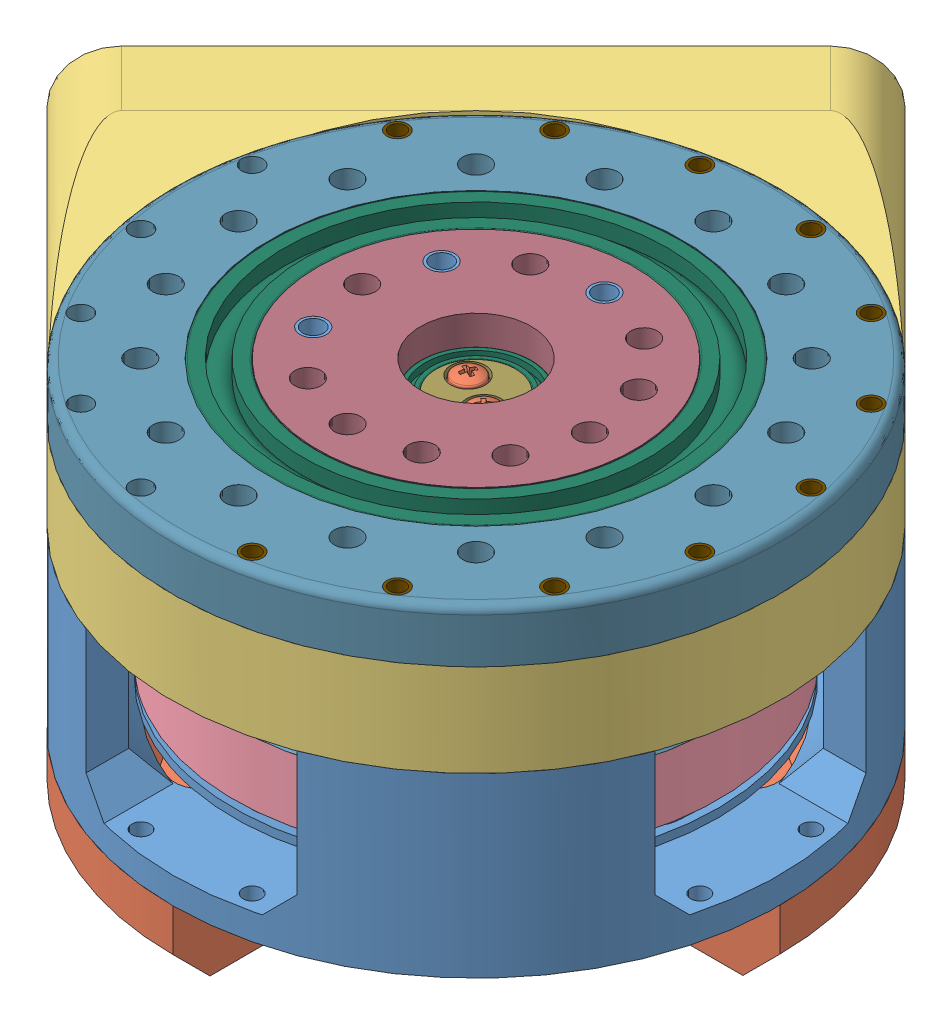
SolidWorks assembly Cycloidal_v2, configuration Default. Lengths in mm. (continued)
Components (placement in the parent): (continued)
- hex nut style 1 gradeab_iso-1: hex nut style 1 gradeab_iso [ISO - 4032 - M3 - W - N] at (47.267 33.7573 119.5643) x (1 0 0) z (0 -1 0) size (5.5 6.35 2.4)
- Cycloidal_Discs_8308-1: Cycloidal_Discs_8308 [Default] at (46.2249 42.227 18.2882) x (0.848672 0 0.528919) z (-0.528919 0 0.848672) size (79.25 5 79.73)
  - Cycloidal_Discs-1: Cycloidal_Discs [Default] at (38.3081 39.5303 58.0959) size (79.25 5 79.73)
  - radial ball bearing_68_iso-1: radial ball bearing_68_iso [ISO 15 RBB - 274 - 14,SI,NC,14_68] at (18.3896 43.2803 46.5959) x (0 1 0) z (0 0 1) size (2.5 7 7)
  - radial ball bearing_68_iso-2: radial ball bearing_68_iso [ISO 15 RBB - 274 - 14,SI,NC,14_68] at (38.3081 43.2803 81.0959) x (0 1 0) z (0 0 1) size (2.5 7 7)
  - radial ball bearing_68_iso-3: radial ball bearing_68_iso [ISO 15 RBB - 274 - 14,SI,NC,14_68] at (18.3896 43.2803 69.5959) x (0 1 0) z (0 0 1) size (2.5 7 7)
  - radial ball bearing_68_iso-4: radial ball bearing_68_iso [ISO 15 RBB - 274 - 14,SI,NC,14_68] at (38.3081 43.2803 35.0959) x (0 1 0) z (0 0 1) size (2.5 7 7)
  - radial ball bearing_68_iso-5: radial ball bearing_68_iso [ISO 15 RBB - 274 - 14,SI,NC,14_68] at (58.2267 43.2803 69.5959) x (0 1 0) z (0 0 1) size (2.5 7 7)
  - radial ball bearing_68_iso-6: radial ball bearing_68_iso [ISO 15 RBB - 274 - 14,SI,NC,14_68] at (58.2267 43.2803 46.5959) x (0 1 0) z (0 0 1) size (2.5 7 7)
- Cycloidal_Discs_8308-2: Cycloidal_Discs_8308 [Default] at (109.8312 37.227 61.5646) x (-0.154095 0 0.988056) z (-0.988056 0 -0.154095) size (79.25 5 79.73)
  - Cycloidal_Discs-1: Cycloidal_Discs [Default] at (38.3081 39.5303 58.0959) size (79.25 5 79.73)
  - radial ball bearing_68_iso-1: radial ball bearing_68_iso [ISO 15 RBB - 274 - 14,SI,NC,14_68] at (18.3896 43.2803 46.5959) x (0 1 0) z (0 0 1) size (2.5 7 7)
  - radial ball bearing_68_iso-2: radial ball bearing_68_iso [ISO 15 RBB - 274 - 14,SI,NC,14_68] at (38.3081 43.2803 81.0959) x (0 1 0) z (0 0 1) size (2.5 7 7)
  - radial ball bearing_68_iso-3: radial ball bearing_68_iso [ISO 15 RBB - 274 - 14,SI,NC,14_68] at (18.3896 43.2803 69.5959) x (0 1 0) z (0 0 1) size (2.5 7 7)
  - radial ball bearing_68_iso-4: radial ball bearing_68_iso [ISO 15 RBB - 274 - 14,SI,NC,14_68] at (38.3081 43.2803 35.0959) x (0 1 0) z (0 0 1) size (2.5 7 7)
  - radial ball bearing_68_iso-5: radial ball bearing_68_iso [ISO 15 RBB - 274 - 14,SI,NC,14_68] at (58.2267 43.2803 69.5959) x (0 1 0) z (0 0 1) size (2.5 7 7)
  - radial ball bearing_68_iso-6: radial ball bearing_68_iso [ISO 15 RBB - 274 - 14,SI,NC,14_68] at (58.2267 43.2803 46.5959) x (0 1 0) z (0 0 1) size (2.5 7 7)
- m6-1: m6 [Default] at (24.3083 92.633 87.7803) x (0 0 -1) z (-1 0 0) size (6 16 6)
- Motor_Cover_v2-2: Motor_Cover_v2 [Default] at (47.267 36.1573 89.1587) x (-1 0 0) z (0 0 -1) size (115 33.6 115)
- driver_cover-1: driver_cover [Default] at (47.267 36.1573 89.1587) x (-0.70834 0 -0.705872) z (-0.705872 0 0.70834) size (81.32 15 115)
- Base_plate_2 _new-1: Base_plate_2 _new [Default] at (47.267 69.6573 89.1587) x (-0.707107 0 0.707107) z (-0.707107 0 -0.707107) size (115 87.5 130)
Mates (geometry in assembly coordinates):
- Coincident1: coincident anti-aligned: plane of motor-X83008S.stp-1/outrunner.stp-1 through (64.3082 69.7573 59.1612) normal (0 1 0); plane of Base_Plate-1 through (47.267 69.7573 89.1587) normal (0 -1 0)
- Concentric1: concentric anti-aligned: line of motor-X83008S.stp-1/outrunner.stp-1 through (54.9232 64.2573 75.6816) axis (0 1 0); cylinder of Base_Plate-1 through (54.9232 76.7573 75.6816) axis (0 -1 0) radius 1.5
- Concentric2: concentric anti-aligned: cylinder of motor-X83008S.stp-1/shaft.stp-1 through (47.267 69.7573 89.1587) axis (0 1 0) radius 1.5; line of Base_Plate-1 through (47.267 76.7573 89.1587) axis (0 -1 0)
- Coincident2: coincident anti-aligned: plane of Base_Plate-1 through (47.267 76.7573 89.1587) normal (0 1 0); plane of Eccentric_Shaft-1/Eccentric_Shaft_bot-1 through (46.5261 76.7573 90.4629) normal (0 -1 0)
- Concentric75: concentric anti-aligned: cylinder of Output_Shaft-1 through (47.267 97.2573 89.1587) axis (0 -1 0) radius 30; cylinder of radial ball bearing_68_iso-39 through (47.267 71.6198 89.1587) axis (0 1 0) radius 30
- Concentric76: concentric anti-aligned: cylinder of Cover-1 through (47.267 97.2573 89.1587) axis (0 -1 0) radius 39; cylinder of radial ball bearing_68_iso-39 through (47.267 71.6198 89.1587) axis (0 1 0) radius 39
- Coincident104: coincident aligned: plane of Cover-1 through (47.267 97.2573 89.1587) normal (0 1 0); plane of radial ball bearing_68_iso-39 through (8.567 97.2573 89.1587) normal (0 1 0)
- Coincident105: coincident aligned: plane of Output_Shaft-1 through (47.267 97.2573 89.1587) normal (0 1 0); plane of Cover-1 through (47.267 97.2573 89.1587) normal (0 1 0)
- Concentric78: concentric anti-aligned: cylinder of Base_Plate-1 through (47.267 76.7573 89.1587) axis (0 -1 0) radius 20; cylinder of radial ball bearing_68_iso-40 through (47.267 52.6198 89.1587) axis (0 1 0) radius 20
- Concentric84: concentric aligned: cylinder of Cover-1 through (15.4472 87.2573 57.3389) axis (0 1 0) radius 2.5; cylinder of m13_bearing-1/m6-1 through (15.4472 86.8573 57.3389) axis (0 1 0) radius 2
- Concentric85: concentric aligned: cylinder of Cover-1 through (47.267 87.2573 134.1587) axis (0 1 0) radius 2.5; cylinder of m13_bearing-11/m6-1 through (47.267 86.8573 134.1587) axis (0 1 0) radius 2
- Concentric86: concentric aligned: cylinder of Cover-1 through (64.4877 87.2573 130.7332) axis (0 1 0) radius 2.5; cylinder of m13_bearing-2/m6-1 through (64.4877 86.8573 130.7332) axis (0 1 0) radius 2
- Concentric87: concentric aligned: cylinder of Cover-1 through (79.0868 87.2573 120.9785) axis (0 1 0) radius 2.5; cylinder of m13_bearing-12/m6-1 through (79.0868 86.8573 120.9785) axis (0 1 0) radius 2
- Concentric88: concentric aligned: cylinder of Cover-1 through (88.8416 87.2573 106.3794) axis (0 1 0) radius 2.5; cylinder of m13_bearing-5/m6-1 through (88.8416 86.8573 106.3794) axis (0 1 0) radius 2
- Concentric89: concentric aligned: cylinder of Cover-1 through (92.267 87.2573 89.1587) axis (0 1 0) radius 2.5; cylinder of m13_bearing-4/m6-1 through (92.267 86.8573 89.1587) axis (0 1 0) radius 2
- Concentric90: concentric aligned: cylinder of Cover-1 through (30.0462 87.2573 47.5841) axis (0 1 0) radius 2.5; cylinder of m13_bearing-6/m6-1 through (30.0462 86.8573 47.5841) axis (0 1 0) radius 2
- Concentric91: concentric aligned: cylinder of Cover-1 through (47.267 87.2573 44.1587) axis (0 1 0) radius 2.5; cylinder of m13_bearing-3/m6-1 through (47.267 86.8573 44.1587) axis (0 1 0) radius 2
- Concentric92: concentric aligned: cylinder of Cover-1 through (64.4877 87.2573 47.5841) axis (0 1 0) radius 2.5; cylinder of m13_bearing-7/m6-1 through (64.4877 86.8573 47.5841) axis (0 1 0) radius 2
- Concentric93: concentric aligned: cylinder of Cover-1 through (79.0868 87.2573 57.3389) axis (0 1 0) radius 2.5; cylinder of m13_bearing-8/m6-1 through (79.0868 86.8573 57.3389) axis (0 1 0) radius 2
- Concentric94: concentric aligned: cylinder of Cover-1 through (88.8416 87.2573 71.9379) axis (0 1 0) radius 2.5; cylinder of m13_bearing-9/m6-1 through (88.8416 86.8573 71.9379) axis (0 1 0) radius 2
- Concentric118: concentric anti-aligned: cylinder of Output_Shaft-1 through (59.94 97.2573 69.965) axis (0 -1 0) radius 2.5; cylinder of M4x6x5.5_brass_insert-1 through (59.94 86.633 69.965) axis (0 1 0) radius 2
- Concentric1211: concentric aligned: cylinder of Cover-1 through (2.3676 97.2573 59.1579) axis (0 -1 0) radius 2; cylinder of M3x4x4.2_brass_insert-2 through (2.3676 92.3553 59.1579) axis (0 -1 0) radius 1.5
- Concentric1221: concentric aligned: cylinder of Cover-1 through (17.2662 97.2573 44.2593) axis (0 -1 0) radius 2; cylinder of M3x4x4.2_brass_insert-3 through (17.2662 92.3553 44.2593) axis (0 -1 0) radius 1.5
- Concentric1251: concentric aligned: cylinder of Cover-1 through (77.2678 97.2573 44.2593) axis (0 -1 0) radius 2; cylinder of M3x4x4.2_brass_insert-6 through (77.2678 92.3553 44.2593) axis (0 -1 0) radius 1.8
- Concentric1271: concentric anti-aligned: cylinder of Cover-1 through (100.2294 97.2573 78.6238) axis (0 -1 0) radius 2; cylinder of M3x4x4.2_brass_insert-8 through (100.2294 98.1594 78.6238) axis (0 1 0) radius 1.8
- Concentric1331: concentric aligned: cylinder of Cover-1 through (36.7321 97.2573 36.1963) axis (0 -1 0) radius 2; cylinder of M3x4x4.2_brass_insert-14 through (36.7321 92.3553 36.1963) axis (0 -1 0) radius 1.8
- Concentric1341: concentric anti-aligned: cylinder of Cover-1 through (57.8019 97.2573 36.1963) axis (0 -1 0) radius 2; cylinder of M3x4x4.2_brass_insert-15 through (57.8019 98.1594 36.1963) axis (0 1 0) radius 2
- Concentric1351: concentric aligned: cylinder of Cover-1 through (92.1663 97.2573 59.1579) axis (0 -1 0) radius 2; cylinder of M3x4x4.2_brass_insert-16 through (92.1663 92.3553 59.1579) axis (0 -1 0) radius 2
- Concentric1361: concentric aligned: cylinder of Cover-1 through (100.2294 97.2573 99.6935) axis (0 -1 0) radius 2; cylinder of M3x4x4.2_brass_insert-17 through (100.2294 92.3553 99.6935) axis (0 -1 0) radius 2
- Concentric1381: concentric aligned: cylinder of Cover-1 through (92.1663 97.2573 119.1595) axis (0 -1 0) radius 2; cylinder of M3x4x4.2_brass_insert-19 through (92.1663 92.3553 119.1595) axis (0 -1 0) radius 2
- Concentric1391: concentric aligned: cylinder of Cover-1 through (77.2678 97.2573 134.058) axis (0 -1 0) radius 2; cylinder of M3x4x4.2_brass_insert-20 through (77.2678 92.3553 134.058) axis (0 -1 0) radius 1.5
- Concentric1401: concentric aligned: cylinder of Cover-1 through (57.8019 97.2573 142.1211) axis (0 -1 0) radius 2; cylinder of M3x4x4.2_brass_insert-21 through (57.8019 92.3553 142.1211) axis (0 -1 0) radius 1.5
- Concentric14041: concentric aligned: cylinder of Output_Shaft-1 through (24.3083 97.2573 87.7803) axis (0 -1 0) radius 2.5; cylinder of M4x6x5.5_brass_insert-6 through (24.3083 80.689 87.7803) axis (0 -1 0) radius 2.5
- Concentric14051: concentric aligned: cylinder of Output_Shaft-1 through (36.9813 97.2573 68.5867) axis (0 -1 0) radius 2.5; cylinder of M4x6x5.5_brass_insert-7 through (36.9813 80.689 68.5867) axis (0 -1 0) radius 2.5
- Concentric14071: concentric aligned: cylinder of Output_Shaft-1 through (48.6453 97.2573 66.2) axis (0 -1 0) radius 2.5; cylinder of M4x6x5.5_brass_insert-9 through (48.6453 85.3133 66.2) axis (0 -1 0) radius 2.5
- Concentric14081: concentric aligned: cylinder of Output_Shaft-1 through (28.0734 97.2573 76.4857) axis (0 -1 0) radius 2.5; cylinder of M4x6x5.5_brass_insert-10 through (28.0734 85.3133 76.4857) axis (0 -1 0) radius 2.5
- Concentric14091: concentric aligned: cylinder of Output_Shaft-1 through (26.695 97.2573 99.4443) axis (0 -1 0) radius 2.5; cylinder of M4x6x5.5_brass_insert-11 through (26.695 85.3133 99.4443) axis (0 -1 0) radius 2.5
- Coincident1438: coincident aligned: plane of M4x6x5.5_brass_insert-1 through (58.0754 92.633 71.6304) normal (0 1 0); plane of M4x6x5.5_brass_insert-6 through (24.3083 92.633 87.7803) normal (0 1 0)
- Coincident1439: coincident aligned: plane of M4x6x5.5_brass_insert-1 through (58.0754 92.633 71.6304) normal (0 1 0); plane of M4x6x5.5_brass_insert-7 through (36.9813 92.633 68.5867) normal (0 1 0)
- Coincident1440: coincident aligned: plane of Output_Shaft-1 through (47.267 97.2573 89.1587) normal (0 1 0); plane of M4x6x5.5_brass_insert-9 through (48.6453 97.2573 66.2) normal (0 1 0)
- Coincident1444: coincident aligned: plane of Output_Shaft-1 through (47.267 97.2573 89.1587) normal (0 1 0); plane of M4x6x5.5_brass_insert-11 through (26.695 97.2573 99.4443) normal (0 1 0)
- Coincident1445: coincident aligned: plane of Output_Shaft-1 through (47.267 97.2573 89.1587) normal (0 1 0); plane of M4x6x5.5_brass_insert-10 through (28.0734 97.2573 76.4857) normal (0 1 0)
- Concentric14151: concentric aligned: cylinder of m13_bearing-2/m6-1 through (64.4877 86.8573 130.7332) axis (0 1 0) radius 2; cylinder of M4x6x5.5_brass_insert-20 through (64.4877 86.8573 130.7332) axis (0 1 0) radius 2
- Concentric14161: concentric aligned: cylinder of m13_bearing-11/m6-1 through (47.267 86.8573 134.1587) axis (0 1 0) radius 2; cylinder of M4x6x5.5_brass_insert-21 through (47.267 86.8573 134.1587) axis (0 1 0) radius 2
- Concentric14171: concentric aligned: cylinder of m13_bearing-1/m6-1 through (15.4472 86.8573 57.3389) axis (0 1 0) radius 2; cylinder of M4x6x5.5_brass_insert-22 through (15.4472 86.8573 57.3389) axis (0 1 0) radius 2
- Concentric14181: concentric aligned: cylinder of m13_bearing-6/m6-1 through (30.0462 86.8573 47.5841) axis (0 1 0) radius 2; cylinder of M4x6x5.5_brass_insert-23 through (30.0462 86.8573 47.5841) axis (0 1 0) radius 2
- Concentric14191: concentric aligned: cylinder of m13_bearing-12/m6-1 through (79.0868 86.8573 120.9785) axis (0 1 0) radius 2; cylinder of M4x6x5.5_brass_insert-24 through (79.0868 98.8014 120.9785) axis (0 1 0) radius 2.3
- Concentric14201: concentric aligned: cylinder of m13_bearing-5/m6-1 through (88.8416 86.8573 106.3794) axis (0 1 0) radius 2; cylinder of M4x6x5.5_brass_insert-25 through (88.8416 86.8573 106.3794) axis (0 1 0) radius 2
- Concentric14211: concentric aligned: cylinder of m13_bearing-4/m6-1 through (92.267 86.8573 89.1587) axis (0 1 0) radius 2; cylinder of M4x6x5.5_brass_insert-26 through (92.267 86.8573 89.1587) axis (0 1 0) radius 2
- Concentric14221: concentric aligned: cylinder of m13_bearing-9/m6-1 through (88.8416 86.8573 71.9379) axis (0 1 0) radius 2; cylinder of M4x6x5.5_brass_insert-27 through (88.8416 86.8573 71.9379) axis (0 1 0) radius 2
- Concentric14241: concentric aligned: cylinder of m13_bearing-7/m6-1 through (64.4877 86.8573 47.5841) axis (0 1 0) radius 2; cylinder of M4x6x5.5_brass_insert-29 through (64.4877 86.8573 47.5841) axis (0 1 0) radius 2
- Concentric14251: concentric aligned: cylinder of m13_bearing-3/m6-1 through (47.267 86.8573 44.1587) axis (0 1 0) radius 2; cylinder of M4x6x5.5_brass_insert-31 through (47.267 86.8573 44.1587) axis (0 1 0) radius 2
- Coincident1447: coincident anti-aligned: plane of m13_bearing-2/m6-1 through (64.4877 86.8573 130.7332) normal (0 1 0); plane of M4x6x5.5_brass_insert-20 through (64.4877 86.8573 130.7332) normal (0 -1 0)
- Coincident1458: coincident aligned: plane of M4x6x5.5_brass_insert-20 through (62.6232 92.8573 132.3986) normal (0 1 0); plane of M4x6x5.5_brass_insert-21 through (45.4024 92.8573 135.824) normal (0 1 0)
- Coincident1459: coincident aligned: plane of M4x6x5.5_brass_insert-20 through (62.6232 92.8573 132.3986) normal (0 1 0); plane of M4x6x5.5_brass_insert-22 through (17.0054 92.8573 59.2938) normal (0 1 0)
- Coincident1460: coincident aligned: plane of M4x6x5.5_brass_insert-20 through (62.6232 92.8573 132.3986) normal (0 1 0); plane of M4x6x5.5_brass_insert-23 through (31.6045 92.8573 49.5391) normal (0 1 0)
- Coincident1461: coincident aligned: plane of M4x6x5.5_brass_insert-20 through (62.6232 92.8573 132.3986) normal (0 1 0); plane of M4x6x5.5_brass_insert-31 through (46.7161 92.8573 46.5972) normal (0 1 0)
- Coincident1462: coincident aligned: plane of M4x6x5.5_brass_insert-20 through (62.6232 92.8573 132.3986) normal (0 1 0); plane of M4x6x5.5_brass_insert-29 through (64.1304 92.8573 50.0584) normal (0 1 0)
- Coincident1463: coincident aligned: plane of M4x6x5.5_brass_insert-20 through (62.6232 92.8573 132.3986) normal (0 1 0); plane of M4x6x5.5_brass_insert-28 through (79.0868 92.8573 57.3389) normal (0 1 0)
- Coincident1464: coincident aligned: plane of M4x6x5.5_brass_insert-20 through (62.6232 92.8573 132.3986) normal (0 1 0); plane of M4x6x5.5_brass_insert-27 through (86.977 92.8573 73.6032) normal (0 1 0)
- Coincident1465: coincident aligned: plane of M4x6x5.5_brass_insert-20 through (62.6232 92.8573 132.3986) normal (0 1 0); plane of M4x6x5.5_brass_insert-26 through (90.4024 92.8573 90.824) normal (0 1 0)
- Coincident1466: coincident aligned: plane of M4x6x5.5_brass_insert-20 through (62.6232 92.8573 132.3986) normal (0 1 0); plane of M4x6x5.5_brass_insert-25 through (86.977 92.8573 108.0448) normal (0 1 0)
- Coincident1467: coincident aligned: plane of M4x6x5.5_brass_insert-20 through (62.6232 92.8573 132.3986) normal (0 1 0); plane of M4x6x5.5_brass_insert-24 through (80.4417 92.8573 123.0795) normal (0 1 0)
- Concentric1426: concentric aligned: cylinder of pan cross head_am-1 through (50.745 118.0573 91.1345) axis (0 1 0) radius 1.5; line of Eccentric_Shaft-1/Eccentric_Shaft_top-1 through (50.745 90.2573 91.1345) axis (0 1 0)
- Coincident1468: coincident anti-aligned: plane of Eccentric_Shaft-1/Eccentric_Shaft_top-1 through (43.789 90.2573 87.1829) normal (0 1 0); plane of pan cross head_am-1 through (51.7391 90.2573 90.0112) normal (0 -1 0)
- Concentric14281: concentric aligned: cylinder of pan cross head_am-3 through (43.789 118.0573 87.1829) axis (0 1 0) radius 2.8; cylinder of Eccentric_Shaft-1/Eccentric_Shaft_top-1 through (43.789 86.7573 87.1829) axis (0 1 0) radius 1.5
- Coincident14701: coincident anti-aligned: plane of Eccentric_Shaft-1/Eccentric_Shaft_top-1 through (50.745 90.2573 91.1345) normal (0 1 0); plane of pan cross head_am-3 through (44.2995 90.2573 85.7724) normal (0 -1 0)
- Concentric1437: concentric anti-aligned: cylinder of Base_Plate-1 through (50.745 76.7573 91.1345) axis (0 -1 0) radius 2; cylinder of M3x4x4.2_brass_insert-22 through (50.745 74.6594 91.1345) axis (0 1 0) radius 1.5
- Coincident1479: coincident aligned: plane of Base_Plate-1 through (47.267 69.7573 89.1587) normal (0 -1 0); plane of M3x4x4.2_brass_insert-22 through (52.2218 69.7573 90.872) normal (0 -1 0)
- Concentric1438: concentric anti-aligned: cylinder of Base_Plate-1 through (43.789 76.7573 87.1829) axis (0 -1 0) radius 2; cylinder of M3x4x4.2_brass_insert-23 through (43.789 74.6594 87.1829) axis (0 1 0) radius 1.5
- Coincident1480: coincident aligned: plane of Base_Plate-1 through (47.267 69.7573 89.1587) normal (0 -1 0); plane of M3x4x4.2_brass_insert-23 through (45.2659 69.7573 86.9207) normal (0 -1 0)
- Concentric1439: concentric anti-aligned: cylinder of Base_Plate-1 through (33.7899 76.7573 81.5025) axis (0 -1 0) radius 1.5; cylinder of pan cross head_am-4 through (33.7899 103.0573 81.5025) axis (0 1 0) radius 1.5
- Coincident1481: coincident anti-aligned: plane of Base_Plate-1 through (33.7899 75.2573 81.5025) normal (0 1 0); plane of pan cross head_am-4 through (35.2899 75.2573 81.5025) normal (0 -1 0)
- Concentric14401: concentric anti-aligned: cylinder of Base_Plate-1 through (60.7441 76.7573 96.8149) axis (0 -1 0) radius 1.5; cylinder of pan cross head_am-5 through (60.7441 103.0573 96.8149) axis (0 1 0) radius 2.8
- Coincident14821: coincident anti-aligned: plane of Base_Plate-1 through (60.7441 75.2573 96.8149) normal (0 1 0); plane of pan cross head_am-5 through (62.2441 75.2573 96.8149) normal (0 -1 0)
- GearMate1: gear = 10 : 1 mm: cylinder of Eccentric_Shaft-1/Eccentric_Shaft_top-1 through (47.267 91.7573 89.1587) axis (0 -1 0) radius 7.5; cylinder of Output_Shaft-1 through (47.267 97.2573 89.1587) axis (0 -1 0) radius 10.5
- Concentric1445021: concentric anti-aligned: cylinder of Base_Plate-1 through (39.6108 76.7573 102.6358) axis (0 -1 0) radius 1.5; cylinder of pan cross head_am-6 through (39.6108 103.0573 102.6358) axis (0 1 0) radius 2.8
- Coincident1486621: coincident anti-aligned: plane of Base_Plate-1 through (39.6108 75.2573 102.6358) normal (0 1 0); plane of pan cross head_am-6 through (41.1108 75.2573 102.6358) normal (0 -1 0)
- Concentric1445031: concentric anti-aligned: cylinder of Base_Plate-1 through (54.9232 76.7573 75.6816) axis (0 -1 0) radius 1.5; cylinder of pan cross head_am-7 through (54.9232 103.0573 75.6816) axis (0 1 0) radius 2.8
- Coincident1486631: coincident anti-aligned: plane of Base_Plate-1 through (54.9232 75.2573 75.6816) normal (0 1 0); plane of pan cross head_am-7 through (56.4232 75.2573 75.6816) normal (0 -1 0)
- Coincident1486632: coincident anti-aligned: plane of Cover-1 through (88.8416 86.8573 71.9379) normal (0 -1 0); plane of m13_bearing-9/radial ball bearing_68_iso-2 through (91.6245 86.8573 68.9955) normal (0 1 0)
- Coincident1486633: coincident anti-aligned: plane of Cover-1 through (88.8416 86.8573 71.9379) normal (0 -1 0); plane of m13_bearing-8/radial ball bearing_68_iso-2 through (78.4447 86.8573 53.3401) normal (0 1 0)
- Coincident1486634: coincident anti-aligned: plane of Cover-1 through (88.8416 86.8573 71.9379) normal (0 -1 0); plane of m13_bearing-7/radial ball bearing_68_iso-2 through (66.6983 86.8573 44.1906) normal (0 1 0)
- Coincident1486635: coincident anti-aligned: plane of Cover-1 through (88.8416 86.8573 71.9379) normal (0 -1 0); plane of m13_bearing-3/radial ball bearing_68_iso-2 through (47.4539 86.8573 40.113) normal (0 1 0)
- Coincident1486636: coincident anti-aligned: plane of Cover-1 through (88.8416 86.8573 71.9379) normal (0 -1 0); plane of m13_bearing-4/radial ball bearing_68_iso-2 through (92.1768 86.8573 85.1097) normal (0 1 0)
- Coincident1486637: coincident anti-aligned: plane of Cover-1 through (88.8416 86.8573 71.9379) normal (0 -1 0); plane of m13_bearing-5/radial ball bearing_68_iso-2 through (88.6021 86.8573 102.3365) normal (0 1 0)
- Coincident1486638: coincident anti-aligned: plane of Cover-1 through (88.8416 86.8573 71.9379) normal (0 -1 0); plane of m13_bearing-12/radial ball bearing_68_iso-2 through (78.3409 86.8573 116.9978) normal (0 1 0)
- Coincident1486639: coincident anti-aligned: plane of Cover-1 through (88.8416 86.8573 71.9379) normal (0 -1 0); plane of m13_bearing-11/radial ball bearing_68_iso-2 through (44.9443 86.8573 130.8409) normal (0 1 0)
- Coincident1486640: coincident anti-aligned: plane of Cover-1 through (88.8416 86.8573 71.9379) normal (0 -1 0); plane of m13_bearing-2/radial ball bearing_68_iso-2 through (64.0006 86.8573 126.7126) normal (0 1 0)
- Coincident1486643: coincident anti-aligned: plane of Cover-1 through (30.0462 86.8573 47.5841) normal (0 -1 0); plane of m13_bearing-6/radial ball bearing_68_iso-2 through (28.2174 86.8573 43.9705) normal (0 1 0)
- Coincident1486644: coincident anti-aligned: plane of Cover-1 through (15.4472 86.8573 57.3389) normal (0 -1 0); plane of m13_bearing-1/radial ball bearing_68_iso-2 through (12.4643 86.8573 54.5994) normal (0 1 0)
- Concentric1445035: concentric anti-aligned: cylinder of Eccentric_Shaft-1/Eccentric_Shaft_bot-1 through (46.5261 81.7573 90.4629) axis (0 -1 0) radius 7.5; cylinder of radial ball bearing_68_iso-46 through (46.5261 59.1198 90.4629) axis (0 1 0) radius 7.5
- Coincident1486648: coincident aligned: plane of Eccentric_Shaft-1/Eccentric_Shaft_bot-1 through (46.5261 81.7573 90.4629) normal (0 1 0); plane of radial ball bearing_68_iso-46 through (38.8261 81.7573 90.4643) normal (0 1 0)
- Concentric1445036: concentric anti-aligned: cylinder of Eccentric_Shaft-1/Eccentric_Shaft_bot-2 through (48.0079 86.7573 87.8544) axis (0 -1 0) radius 7.5; cylinder of radial ball bearing_68_iso-44 through (48.0079 64.1198 87.8544) axis (0 1 0) radius 7.5
- Coincident1486649: coincident aligned: plane of Eccentric_Shaft-1/Eccentric_Shaft_bot-2 through (48.0079 82.7573 87.8544) normal (0 1 0); circle of radial ball bearing_68_iso-44
- Concentric1445037: concentric anti-aligned: cylinder of Eccentric_Shaft-1/Eccentric_Shaft_top-1 through (47.267 91.7573 89.1587) axis (0 -1 0) radius 7.5; cylinder of radial ball bearing_68_iso-45 through (47.267 69.1198 89.1587) axis (0 1 0) radius 7.5
- Concentric1445038: concentric anti-aligned: cylinder of Base_Plate-1 through (47.267 76.7573 89.1587) axis (0 -1 0) radius 20; cylinder of radial ball bearing_68_iso-40 through (47.267 52.6198 89.1587) axis (0 1 0) radius 20
- Coincident1486655: coincident anti-aligned: plane of Eccentric_Shaft-1/Eccentric_Shaft_top-1 through (47.267 87.7573 89.1587) normal (0 1 0); plane of radial ball bearing_68_iso-45 through (47.5372 87.7573 97.5543) normal (0 -1 0)
- Concentric1445042: concentric anti-aligned: cylinder of Base_Plate-1 through (43.789 76.7573 87.1829) axis (0 -1 0) radius 2; cylinder of Eccentric_Shaft-1/Eccentric_Shaft_bot-1 through (43.789 76.7573 87.1829) axis (0 1 0) radius 1.5
- Concentric1445043: concentric aligned: cylinder of Eccentric_Shaft-1/Eccentric_Shaft_bot-1 through (50.745 76.7573 91.1345) axis (0 1 0) radius 1.5; cylinder of M3x4x4.2_brass_insert-22 through (50.745 74.6594 91.1345) axis (0 1 0) radius 1.5
- Coincident1486660: coincident aligned: plane of Cover-1 through (5.6924 86.8573 71.9379) normal (0 -1 0); circle of m13_bearing-31/radial ball bearing_68_iso-2
- Coincident1486661: coincident aligned: plane of Cover-1 through (5.6924 86.8573 71.9379) normal (0 -1 0); circle of m13_bearing-32/radial ball bearing_68_iso-2
- Coincident1486662: coincident aligned: plane of Cover-1 through (5.6924 86.8573 71.9379) normal (0 -1 0); circle of m13_bearing-36/radial ball bearing_68_iso-2
- Coincident1486663: coincident aligned: plane of Cover-1 through (5.6924 86.8573 71.9379) normal (0 -1 0); circle of m13_bearing-35/radial ball bearing_68_iso-2
- Coincident1486664: coincident aligned: plane of Cover-1 through (5.6924 86.8573 71.9379) normal (0 -1 0); circle of m13_bearing-34/radial ball bearing_68_iso-2
- Concentric1445052: concentric aligned: circle of m13_bearing-31/m6-1; cylinder of M4x6x5.5_brass_insert-47 through (5.6924 92.8573 71.9379) axis (0 -1 0) radius 2
- Concentric14450531: concentric aligned: line of Cover-1 through (5.6924 86.8573 106.3794) axis (0 1 0); cylinder of M4x6x5.5_brass_insert-49 through (5.6924 87.0073 106.3794) axis (0 1 0) radius 2
- Concentric14450541: concentric aligned: line of Cover-1 through (15.4472 86.8573 120.9785) axis (0 1 0); cylinder of M4x6x5.5_brass_insert-50 through (15.4472 86.8573 120.9785) axis (0 1 0) radius 2
- Concentric1445056: concentric aligned: circle of m13_bearing-32/m6-1; cylinder of M4x6x5.5_brass_insert-48 through (2.267 92.8573 89.1587) axis (0 -1 0) radius 2
- Coincident1486681: coincident anti-aligned: plane of m13_bearing-1/m6-1 through (15.4472 92.8573 57.3389) normal (0 1 0); circle of M4x6x5.5_brass_insert-47
- Concentric1445063: concentric aligned: cylinder of m13_bearing-34/m6-1 through (30.0462 87.0073 130.7332) axis (0 1 0) radius 2; cylinder of M4x6x5.5_brass_insert-51 through (30.0462 87.0073 130.7332) axis (0 1 0) radius 2
- Coincident1486686: coincident aligned: plane of m13_bearing-36/m6-1 through (5.6924 93.0073 106.3794) normal (0 1 0); circle of M4x6x5.5_brass_insert-49
- Coincident1486687: coincident anti-aligned: plane of m13_bearing-32/m6-1 through (2.267 92.8573 89.1587) normal (0 1 0); circle of M4x6x5.5_brass_insert-48
- Coincident1486688: coincident aligned: plane of m13_bearing-35/m6-1 through (15.4472 92.8573 120.9785) normal (0 1 0); circle of M4x6x5.5_brass_insert-50
- Coincident1486690: coincident aligned: plane of m13_bearing-34/m6-1 through (30.0462 93.0073 130.7332) normal (0 1 0); circle of M4x6x5.5_brass_insert-51
- Coincident1486692: coincident anti-aligned: plane of foc-motor-controller.step-1/foc-motor-controller_PCB.step-1 through (47.267 33.7573 89.1587) normal (0 1 0); plane of hex nut style 1 gradeab_iso-1 through (47.267 33.7573 122.7397) normal (0 -1 0)
- Concentric14450545: concentric anti-aligned: cylinder of radial ball bearing_68_iso-46 through (46.5261 59.1198 90.4629) axis (0 1 0) radius 10.5; cylinder of Cycloidal_Discs_8308-2/Cycloidal_Discs-1 through (46.5261 81.7573 90.4629) axis (0 -1 0) radius 10.5
- Coincident1486693: coincident aligned: plane of radial ball bearing_68_iso-46 through (36.2261 81.7573 90.4647) normal (0 1 0); plane of Cycloidal_Discs_8308-2/Cycloidal_Discs-1 through (84.4035 81.7573 96.5395) normal (0 1 0)
- Concentric14450546: concentric anti-aligned: cylinder of radial ball bearing_68_iso-44 through (48.0079 64.1198 87.8544) axis (0 1 0) radius 10.5; cylinder of Cycloidal_Discs_8308-1/Cycloidal_Discs-1 through (48.0079 86.7573 87.8544) axis (0 -1 0) radius 10.5
- Coincident1486694: coincident aligned: plane of radial ball bearing_68_iso-44 through (55.2094 86.7573 80.4904) normal (0 1 0); plane of Cycloidal_Discs_8308-1/Cycloidal_Discs-1 through (68.44 86.7573 55.3867) normal (0 1 0)
- Concentric14450547: concentric anti-aligned: cylinder of M4x6x5.5_brass_insert-6 through (24.3083 92.633 87.7803) axis (0 -1 0) radius 2; cylinder of m6-1 through (24.3083 86.633 87.7803) axis (0 1 0) radius 2
- Coincident1486695: coincident anti-aligned: circle of M4x6x5.5_brass_insert-6; plane of m6-1 through (24.3083 86.633 87.7803) normal (0 1 0)
- Tangent1: tangent aligned: cylinder of Cycloidal_Discs_8308-1/radial ball bearing_68_iso-3 through (25.021 64.8698 87.0788) axis (0 1 0) radius 2; cylinder of m6-1 through (24.3083 76.633 87.7803) axis (0 1 0) radius 3
- Tangent3: tangent aligned: cylinder of Cycloidal_Discs_8308-2/radial ball bearing_68_iso-2 through (23.8008 59.8698 86.9187) axis (0 1 0) radius 2; cylinder of m6-1 through (24.3083 76.633 87.7803) axis (0 1 0) radius 3
- Concentric14450553: concentric aligned: cylinder of Cover-1 through (47.267 97.2573 89.1587) axis (0 -1 0) radius 57.5; cylinder of Motor_Cover_v2-2 through (47.267 69.7573 89.1587) axis (0 -1 0) radius 57.5
- Concentric14450559: concentric anti-aligned: cylinder of foc-motor-controller.step-1/foc-motor-controller_PCB.step-1 through (47.267 33.8033 58.7531) axis (0 1 0) radius 1.6; cylinder of Motor_Cover_v2-2 through (47.267 86.1573 58.7531) axis (0 -1 0) radius 1.5
- Concentric14450560: concentric anti-aligned: circle of foc-motor-controller.step-1/foc-motor-controller_PCB.step-1; cylinder of Motor_Cover_v2-2 through (47.267 86.1573 119.5643) axis (0 -1 0) radius 1.5
- Coincident1486699: coincident anti-aligned: line of foc-motor-controller.step-1/foc-motor-controller_PCB.step-1 through (47.267 32.2473 119.5643) axis (0 1 0); line of hex nut style 1 gradeab_iso-1 through (47.267 35.9569 119.5643) axis (0 -1 0)
- Coincident1486700: coincident aligned: circle of hex nut style 1 gradeab_iso-1; plane of Motor_Cover_v2-2 through (47.267 36.1573 89.1587) normal (0 -1 0)
- Concentric14450561: concentric anti-aligned: cylinder of Motor_Cover_v2-2 through (47.267 69.7573 89.1587) axis (0 -1 0) radius 57.5; cylinder of driver_cover-1 through (47.267 21.1573 89.1587) axis (0 1 0) radius 57.5
- Coincident1486701: coincident anti-aligned: plane of Motor_Cover_v2-2 through (47.267 36.1573 89.1587) normal (0 -1 0); plane of driver_cover-1 through (47.267 36.1573 89.1587) normal (0 1 0)
- Concentric14450563: concentric aligned: cylinder of Cover-1 through (47.267 97.2573 89.1587) axis (0 -1 0) radius 57.5; cylinder of Base_plate_2 _new-1 through (47.267 76.6573 89.1587) axis (0 -1 0) radius 57.5
- Coincident1486702: coincident aligned: circle of Cover-1; plane of Base_plate_2 _new-1 through (47.267 87.2573 89.1587) normal (0 1 0)
- Concentric14450564: concentric aligned: cylinder of m13_bearing-36/radial ball bearing_68_iso-2 through (5.6924 105.1448 106.3794) axis (0 -1 0) radius 6.5; cylinder of Base_plate_2 _new-1 through (5.6924 87.2573 106.3794) axis (0 -1 0) radius 7
- Concentric14450565: concentric aligned: cylinder of m13_bearing-36/m6-1 through (5.6924 87.0073 106.3794) axis (0 1 0) radius 2; cylinder of M4x6x5.5_brass_insert-49 through (5.6924 87.0073 106.3794) axis (0 1 0) radius 2
- Coincident1486703: coincident anti-aligned: plane of Motor_Cover_v2-2 through (47.267 69.7573 89.1587) normal (0 1 0); plane of Base_plate_2 _new-1 through (47.267 69.7573 89.1587) normal (0 -1 0)
- Concentric14450566: concentric aligned: cylinder of Motor_Cover_v2-2 through (77.2678 86.1573 44.2593) axis (0 -1 0) radius 1.75; cylinder of driver_cover-1 through (77.2678 36.1573 44.2593) axis (0 -1 0) radius 1.75
- Concentric14450567: concentric aligned: cylinder of Motor_Cover_v2-2 through (77.2678 86.1573 134.058) axis (0 -1 0) radius 1.75; line of Base_plate_2 _new-1 through (77.2678 87.2573 134.058) axis (0 -1 0)
- Concentric14450568: concentric anti-aligned: cylinder of radial ball bearing_68_iso-40 through (47.267 52.6198 89.1587) axis (0 1 0) radius 26; cylinder of Base_plate_2 _new-1 through (47.267 76.6573 89.1587) axis (0 -1 0) radius 26
- Coincident1486704: coincident aligned: plane of radial ball bearing_68_iso-40 through (23.0716 69.7573 88.686) normal (0 -1 0); plane of Base_plate_2 _new-1 through (47.267 69.7573 89.1587) normal (0 -1 0)
- Concentric14450569: concentric anti-aligned: cylinder of Base_Plate-1 through (47.267 76.7573 89.1587) axis (0 -1 0) radius 20; cylinder of radial ball bearing_68_iso-40 through (47.267 52.6198 89.1587) axis (0 1 0) radius 20
- Coincident1486705: coincident aligned: circle of motor-X83008S.stp-1/outrunner.stp-1; plane of Base_plate_2 _new-1 through (47.267 69.7573 89.1587) normal (0 -1 0)
